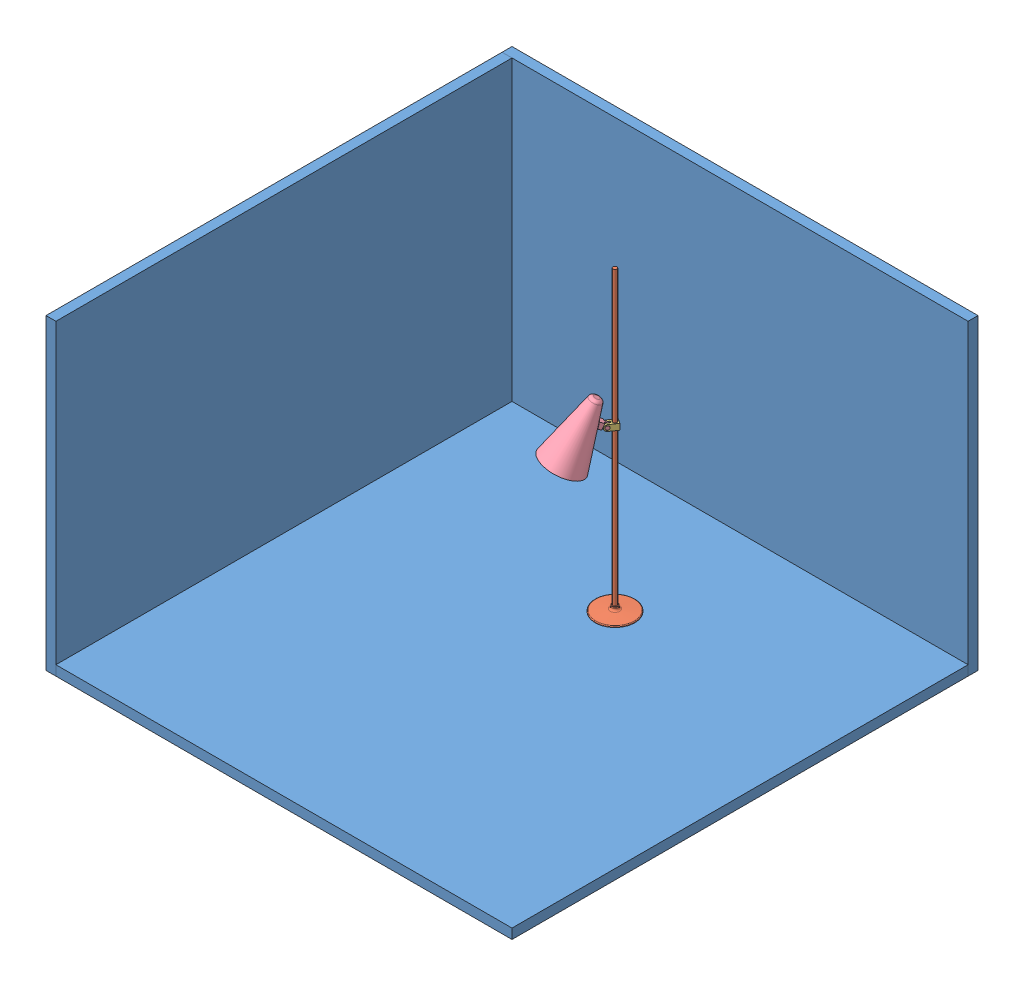
SolidWorks assembly Render Assembly, configuration Default. Lengths in mm.
Overall size (2350 1550 2350).
4 component instances, 4 part files, 6 mates.
Components (placement in the parent):
- Background for Render-1: Background for Render [Default] at (-1172.3978 -723.4798 -1101.0217) size (2350 1550 2350)
- Lamp Base-1: Lamp Base [Default] at (4.5509 -723.4798 -443.4759) size (200 1500 200)
- Lamp Clamp-1: Lamp Clamp [Default] at (4.5509 91.5202 -443.4759) x (0.565217 0 -0.824942) z (0.824942 0 0.565217) size (60 30 30)
- Lamp Shade-1: Lamp Shade [Default] at (-104.7465 -52.9735 -283.9548) x (0.51226 -0.422618 -0.747652) z (0.824942 0 0.565217) size (203.94 302 203.88)
Mates (geometry in assembly coordinates):
- Coincident1: coincident anti-aligned: plane of Background for Render-1 through (-1172.3978 -723.4798 -1101.0217) normal (0 1 0); plane of Lamp Base-1 through (4.5509 -723.4798 -443.4759) normal (0 -1 0)
- Concentric1: concentric anti-aligned: cylinder of Lamp Base-1 through (4.5509 -723.4798 -443.4759) axis (0 1 0) radius 10; cylinder of Lamp Clamp-1 through (4.5509 106.5202 -443.4759) axis (0 -1 0) radius 10
- Concentric2: concentric anti-aligned: cylinder of Lamp Clamp-1 through (-24.7798 91.5202 -427.2059) axis (0.824942 0 0.565217) radius 10; cylinder of Lamp Shade-1 through (-0.0315 91.5202 -410.2494) axis (-0.824942 0 -0.565217) radius 10
- Coincident2: coincident anti-aligned: plane of Lamp Clamp-1 through (-25.0086 106.5202 -409.1796) normal (0.824942 0 0.565217); plane of Lamp Shade-1 through (-16.5303 91.5202 -421.5537) normal (-0.824942 0 -0.565217)
- Distance1: distance = 800 mm anti-aligned: plane of Background for Render-1 through (-1172.3978 -723.4798 -1101.0217) normal (0 1 0); plane of Lamp Clamp-1 through (4.5509 76.5202 -443.4759) normal (0 -1 0)
- Angle2: planar angle = 0.436332 rad aligned: plane of Lamp Clamp-1 through (4.5509 106.5202 -443.4759) normal (0 1 0); plane of Lamp Shade-1 through (-256171.1865 211451.0135 373475.444) normal (0.238871 0.906308 -0.348636)
